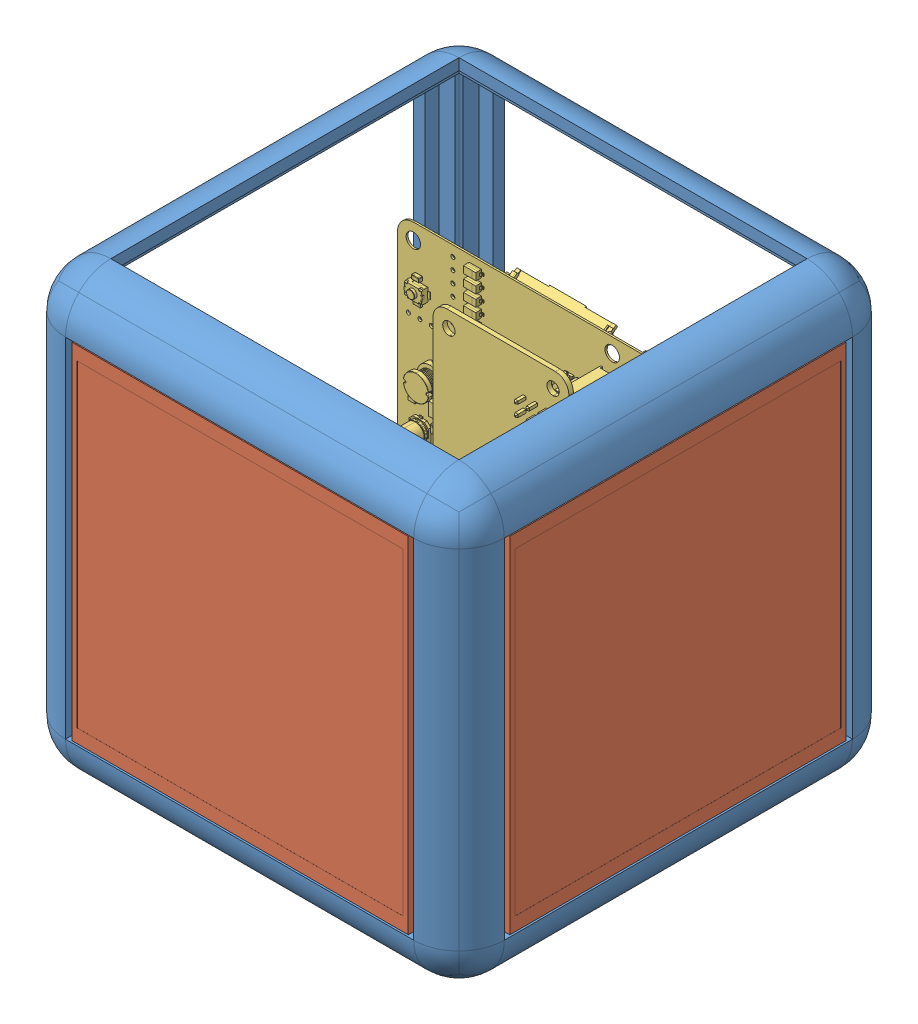
SolidWorks assembly Cube, configuration По умолчанию. Lengths in mm.
Overall size (96.86 96.86 96.86).
9 component instances, 3 part files, 16 mates.
Components (placement in the parent):
- Frame-1: Frame [По умолчанию] at (51.086 82.6322 12.8914) size (6.46 91 91)
- Frame-2: Frame [По умолчанию] at (44.0149 82.6322 96.8203) x (0 0 -1) z (1 0 0) size (6.46 91 91)
- Frame-5: Frame [По умолчанию] at (135.0149 82.6322 19.9625) x (0 0 1) z (-1 0 0) size (6.46 91 91)
- Frame-6: Frame [По умолчанию] at (127.9439 82.6322 103.8914) x (-1 0 0) z (0 0 -1) size (6.46 91 91)
- Frame-7: Frame [По умолчанию] at (51.086 82.6322 103.8914) x (0 -1 0) z (0 0 -1) size (6.46 91 91)
- Frame-8: Frame [По умолчанию] at (127.9439 5.7744 103.8914) x (0 1 0) z (0 0 -1) size (6.46 91 91)
- Display-4: Display [По умолчанию] at (89.5149 44.2033 103.3203) size (83 83 3.41)
- Display-5: Display [По умолчанию] at (134.4439 44.2033 58.3914) x (0 0 -1) z (1 0 0) size (83 83 3.41)
- SmartCube-2: SmartCube [По умолчанию] at (57.6334 11.2906 40.0916) size (65 65.1 40.65)
Mates (geometry in assembly coordinates):
- Совпадение1: coincident anti-aligned: plane of Frame-1 through (51.086 89.7033 96.8203) normal (0.707107 0 0.707107); plane of Frame-2 through (51.086 -1.2967 96.8203) normal (-0.707107 0 -0.707107)
- Совпадение2: coincident anti-aligned: line of Frame-1 through (47.5505 86.1677 100.3559) axis (-0.57735 0.57735 0.57735); line of Frame-2 through (45.3125 88.4057 102.5938) axis (0.57735 -0.57735 -0.57735)
- Совпадение3: coincident aligned: line of Frame-1 through (45.3125 0.0008 102.5938) axis (0.57735 0.57735 -0.57735); line of Frame-2 through (45.3125 0.0008 102.5938) axis (0.57735 0.57735 -0.57735)
- Совпадение7: coincident anti-aligned: plane of Frame-5 through (127.9439 -1.2967 19.9625) normal (0.707107 0 0.707107); plane of Frame-6 through (127.9439 89.7033 19.9625) normal (-0.707107 0 -0.707107)
- Совпадение8: coincident anti-aligned: line of Frame-5 through (133.7174 88.4057 14.189) axis (-0.57735 -0.57735 0.57735); line of Frame-6 through (131.4794 86.1677 16.4269) axis (0.57735 0.57735 -0.57735)
- Совпадение9: coincident aligned: line of Frame-5 through (133.7174 0.0008 14.189) axis (-0.57735 0.57735 0.57735); line of Frame-6 through (133.7174 0.0008 14.189) axis (-0.57735 0.57735 0.57735)
- Совпадение10: coincident anti-aligned: line of Frame-2 through (131.4794 86.1677 100.3559) axis (0.57735 0.57735 0.57735); line of Frame-6 through (133.7174 88.4057 102.5938) axis (-0.57735 -0.57735 -0.57735)
- Совпадение11: coincident aligned: line of Frame-2 through (133.7174 0.0008 102.5938) axis (-0.57735 0.57735 -0.57735); line of Frame-6 through (133.7174 0.0008 102.5938) axis (-0.57735 0.57735 -0.57735)
- Совпадение12: coincident aligned: line of Frame-2 through (45.3125 88.4057 102.5938) axis (0.57735 -0.57735 -0.57735); line of Frame-7 through (45.3125 88.4057 102.5938) axis (0.57735 -0.57735 -0.57735)
- Совпадение13: coincident aligned: line of Frame-6 through (133.7174 88.4057 102.5938) axis (-0.57735 -0.57735 -0.57735); line of Frame-7 through (133.7174 88.4057 102.5938) axis (-0.57735 -0.57735 -0.57735)
- Совпадение14: coincident anti-aligned: line of Frame-5 through (133.7174 0.0008 14.189) axis (-0.57735 0.57735 0.57735); line of Frame-8 through (131.4794 2.2388 16.4269) axis (0.57735 -0.57735 -0.57735)
- Совпадение15: coincident aligned: line of Frame-2 through (45.3125 0.0008 102.5938) axis (0.57735 0.57735 -0.57735); line of Frame-8 through (45.3125 0.0008 102.5938) axis (0.57735 0.57735 -0.57735)
- Совпадение31: coincident aligned: line of Frame-2 through (48.0149 85.7033 104.3203) axis (1 0 0); line of Display-4 through (48.0149 85.7033 104.3203) axis (1 0 0)
- Совпадение32: coincident anti-aligned: line of Frame-2 through (131.0149 85.7033 104.3203) axis (0 -1 0); line of Display-4 through (131.0149 2.7033 104.3203) axis (0 1 0)
- Совпадение34: coincident aligned: line of Frame-6 through (135.4439 85.7033 99.8914) axis (0 0 -1); line of Display-5 through (135.4439 85.7033 99.8914) axis (0 0 -1)
- Совпадение35: coincident anti-aligned: line of Frame-6 through (135.4439 85.7033 16.8914) axis (0 -1 0); line of Display-5 through (135.4439 2.7033 16.8914) axis (0 1 0)
